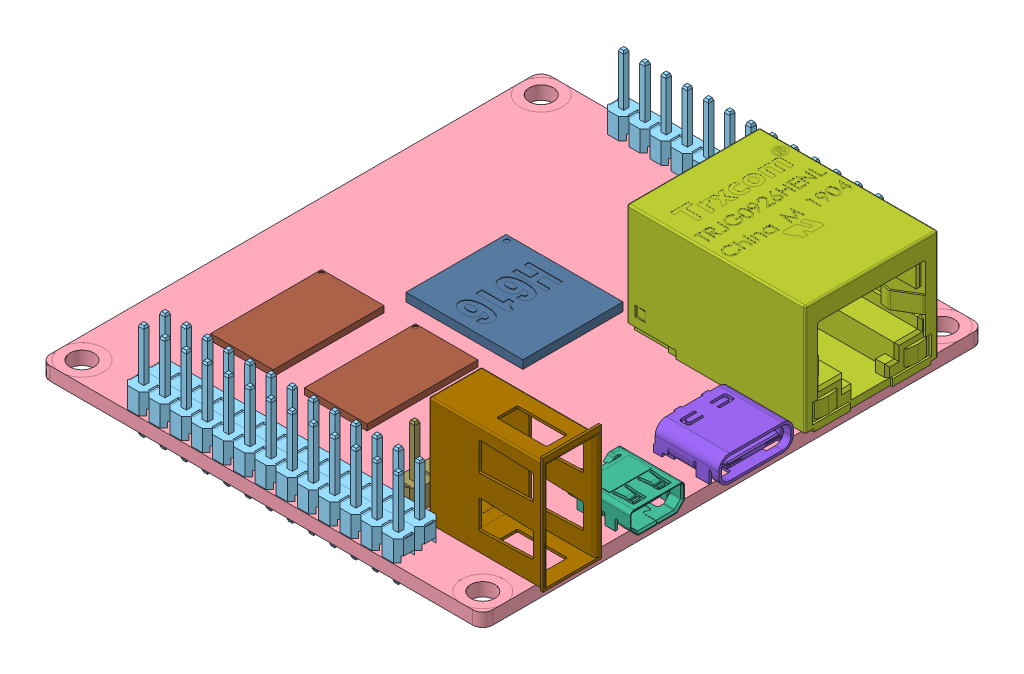
SolidWorks assembly OrangePi_Zero2, configuration 默认. Lengths in mm.
Overall size (54.2 18.1 60).
16 component instances, 12 part files, 37 mates.
Components (placement in the parent):
- Card slot assembly_Domyslna^OrangePi_Zero2-1: Card slot assembly_Domyslna^OrangePi_Zero2 [默认] at (-29.7448 -12.71 -17.6643) x (0 0 -1) z (0 1 0) size (11.95 11.4 1.48) (virtual)
  - card slot part 2 metal pin_Domyslna^Card slot assembly_Domyslna_OrangePi_Zero2-1: card slot part 2 metal pin_Domyslna^Card slot assembly_Domyslna_OrangePi_Zero2 [默认] at (-3.5293 -7.6678 12.2938) x (0 -1 0) z (1 0 0) size (7.95 0.89 8.04) (virtual)
  - sd card slot v1_Domyslna^Card slot assembly_Domyslna_OrangePi_Zero2-1: sd card slot v1_Domyslna^Card slot assembly_Domyslna_OrangePi_Zero2 [默认] at (-18.1743 -9.7848 12.71) x (-1 0 0) z (0 0 -1) size (11.71 10.28 1.3) (virtual)
  - part 3 v1_Domyslna^Card slot assembly_Domyslna_OrangePi_Zero2-1: part 3 v1_Domyslna^Card slot assembly_Domyslna_OrangePi_Zero2 [默认] at (-6.4643 -9.3448 11.38) x (1 0 0) z (0 0 -1) size (11.95 11.4 1.45) (virtual)
- pcb^OrangePi_Zero2-1: pcb^OrangePi_Zero2 [默认] at origin size (53 1.6 60) (virtual)
- PLS-13.step^OrangePi_Zero2-1: PLS-13.step^OrangePi_Zero2 [默认] at (-15.45 1.6 26.09) x (1 0 0) z (0 1 0) size (33.02 2.54 11.6) (virtual)
- PLS-13.step^OrangePi_Zero2-2: PLS-13.step^OrangePi_Zero2 [默认] at (-15.45 1.6 28.63) x (1 0 0) z (0 1 0) size (33.02 2.54 11.6) (virtual)
- PLS-13.step^OrangePi_Zero2-3: PLS-13.step^OrangePi_Zero2 [默认] at (-15.25 1.6 -28.63) x (1 0 0) z (0 1 0) size (33.02 2.54 11.6) (virtual)
- 11.0 Female micro HDMI connector_Domyslna^OrangePi_Zero2-1: 11.0 Female micro HDMI connector_Domyslna^OrangePi_Zero2 [默认] at (20 3.05 10.09) x (0 0 -1) z (1 0 0) size (6.5 3.51 7.5) (virtual)
- 12.0 Gigabit ethernet port raspberry^OrangePi_Zero2-1: 12.0 Gigabit ethernet port raspberry^OrangePi_Zero2 [默认] at (27.3 8.525 -15.75) x (0 0 -1) z (1 0 0) size (16.1 17.2 21.45) (virtual)
- 10.0 Female USB connector_Domyslna^OrangePi_Zero2-1: 10.0 Female USB connector_Domyslna^OrangePi_Zero2 [默认] at (19.99 3.18 -1.63) x (0 0 -1) z (1 0 0) size (8.94 3.96 7.9) (virtual)
- USB-A 111 (vertical on plate)___ _________^OrangePi_Zero2-1: USB-A 111 (vertical on plate)___ _________^OrangePi_Zero2 [默认] at (13.7 8.1368 23.65) x (1 0 0) z (0 1 0) size (14 9.14 18.1) (virtual)
- H616^OrangePi_Zero2-1: H616^OrangePi_Zero2 [默认] at (-3.5 1.72 -3.8) x (0 0 1) z (-1 0 0) size (12 1.12 14) (virtual)
- DDR3^OrangePi_Zero2-1: DDR3^OrangePi_Zero2 [默认] at (-14.25 1.9 11.45) size (7.5 1.03 13.3) (virtual)
- DDR3^OrangePi_Zero2-2: DDR3^OrangePi_Zero2 [默认] at (-3.01 1.9 11.45) size (7.5 1.03 13.3) (virtual)
- PLS-4^OrangePi_Zero2-1: PLS-4^OrangePi_Zero2 [默认] at (10.73 1.6 17.31) x (0 0 1) z (0 1 0) size (7.62 2.54 11.6) (virtual)
Mates (geometry in assembly coordinates):
- 重合1: coincident: plane of pcb^OrangePi_Zero2-1 through (0 1.6 0) normal (0 1 0); plane of 12.0 Gigabit ethernet port raspberry^OrangePi_Zero2-1 through (27.3 1.6 -15.75) normal (0 -1 0)
- 距离1: distance = 0.8 mm: plane of 12.0 Gigabit ethernet port raspberry^OrangePi_Zero2-1 through (27.3 8.525 -15.75) normal (1 0 0); plane of pcb^OrangePi_Zero2-1 through (26.5 1.6 -30) normal (1 0 0)
- 距离2: distance = 6.3 mm: plane of pcb^OrangePi_Zero2-1 through (27.25 1.4 -30) normal (0 0 -1); plane of 12.0 Gigabit ethernet port raspberry^OrangePi_Zero2-1 through (5.95 1.95 -23.7) normal (0 0 -1)
- 重合2: coincident: plane of pcb^OrangePi_Zero2-1 through (0 1.6 0) normal (0 1 0); plane of 10.0 Female USB connector_Domyslna^OrangePi_Zero2-1 through (27.6 1.6 1.54) normal (0 -1 0)
- 距离3: distance = 1.1 mm: plane of 10.0 Female USB connector_Domyslna^OrangePi_Zero2-1 through (27.6 3.46 1.54) normal (1 0 0); plane of pcb^OrangePi_Zero2-1 through (26.5 1.6 -30) normal (1 0 0)
- 距离4: distance = 23.9 mm: plane of pcb^OrangePi_Zero2-1 through (27.25 1.4 -30) normal (0 0 -1); plane of 10.0 Female USB connector_Domyslna^OrangePi_Zero2-1 through (27.6 2.9 -6.1) normal (0 0 -1)
- 重合4: coincident: plane of pcb^OrangePi_Zero2-1 through (0 1.6 0) normal (0 1 0); plane of 11.0 Female micro HDMI connector_Domyslna^OrangePi_Zero2-1 through (22 1.6 7.3221) normal (0 -1 0)
- 重合5: coincident: plane of pcb^OrangePi_Zero2-1 through (0 1.6 0) normal (0 1 0); plane of 11.0 Female micro HDMI connector_Domyslna^OrangePi_Zero2-1 through (22 1.6 7.3221) normal (0 -1 0)
- 距离5: distance = 1 mm: plane of 11.0 Female micro HDMI connector_Domyslna^OrangePi_Zero2-1 through (27.5 2.05 12.2455) normal (1 0 0); plane of pcb^OrangePi_Zero2-1 through (26.5 1.6 -30) normal (1 0 0)
- 距离6: distance = 4 mm: plane of 10.0 Female USB connector_Domyslna^OrangePi_Zero2-1 through (27.6 3.46 2.84) normal (0 0 1); plane of 11.0 Female micro HDMI connector_Domyslna^OrangePi_Zero2-1 through (27.5 2.7298 6.84) normal (0 0 -1)
- 重合7: coincident: plane of pcb^OrangePi_Zero2-1 through (0 1.6 0) normal (0 1 0); plane of USB-A 111 (vertical on plate)___ _________^OrangePi_Zero2-1 through (17.9 1.6 16) normal (0 -1 0)
- 距离7: distance = 1.2 mm: plane of USB-A 111 (vertical on plate)___ _________^OrangePi_Zero2-1 through (27.7 1.5868 17.35) normal (1 0 0); plane of pcb^OrangePi_Zero2-1 through (26.5 1.6 -30) normal (1 0 0)
- 距离8: distance = 6.35 mm: plane of USB-A 111 (vertical on plate)___ _________^OrangePi_Zero2-1 through (13.7 1.5868 23.65) normal (0 0 1); plane of pcb^OrangePi_Zero2-1 through (27.25 1.4 30) normal (0 0 1)
- 重合8: coincident: plane of Card slot assembly_Domyslna^OrangePi_Zero2-1/sd card slot v1_Domyslna^Card slot assembly_Domyslna_OrangePi_Zero2-1 through (-24.6 0 -5.98) normal (0 1 0); plane of pcb^OrangePi_Zero2-1 through (0 0 0) normal (0 -1 0)
- 距离9: distance = 0.4 mm: plane of Card slot assembly_Domyslna^OrangePi_Zero2-1/part 3 v1_Domyslna^Card slot assembly_Domyslna_OrangePi_Zero2-1 through (-26.1 -1.45 -17.175) normal (-1 0 0); plane of pcb^OrangePi_Zero2-1 through (-26.5 1.6 -30) normal (-1 0 0)
- 距离11: distance = 12.825 mm: plane of Card slot assembly_Domyslna^OrangePi_Zero2-1/part 3 v1_Domyslna^Card slot assembly_Domyslna_OrangePi_Zero2-1 through (-26.1 -1.45 -17.175) normal (0 0 -1); plane of pcb^OrangePi_Zero2-1 through (27.25 1.4 -30) normal (0 0 -1)
- 重合11: coincident: plane of pcb^OrangePi_Zero2-1 through (0 1.6 0) normal (0 1 0); plane of PLS-13.step^OrangePi_Zero2-3 through (-12.71 1.6 -28.63) normal (0 -1 0)
- 重合13: coincident: plane of PLS-13.step^OrangePi_Zero2-1 through (-12.91 1.6 26.09) normal (0 -1 0); plane of PLS-13.step^OrangePi_Zero2-2 through (-12.91 1.6 28.63) normal (0 -1 0)
- 重合14: coincident: plane of PLS-13.step^OrangePi_Zero2-1 through (14.36 1.6 27.36) normal (0 0 1); plane of PLS-13.step^OrangePi_Zero2-2 through (15.7 1.6 27.36) normal (0 0 -1)
- 重合15: coincident: plane of PLS-13.step^OrangePi_Zero2-1 through (16.3 1.6 26.76) normal (1 0 0); plane of PLS-13.step^OrangePi_Zero2-2 through (16.3 1.6 29.3) normal (1 0 0)
- 重合16: coincident: plane of pcb^OrangePi_Zero2-1 through (0 1.6 0) normal (0 1 0); plane of PLS-13.step^OrangePi_Zero2-2 through (-12.91 1.6 28.63) normal (0 -1 0)
- 对称1: symmetric: plane of PLS-13.step^OrangePi_Zero2-2 through (14.36 1.6 29.9) normal (0 0 1); plane of PLS-13.step^OrangePi_Zero2-3 through (15.9 1.6 -29.9) normal (0 0 -1); plane of assembly
- 距离12: distance = 59.8 mm: plane of PLS-13.step^OrangePi_Zero2-3 through (15.9 1.6 -29.9) normal (0 0 -1); plane of PLS-13.step^OrangePi_Zero2-2 through (14.36 1.6 29.9) normal (0 0 1)
- 距离13: distance = 10 mm: plane of PLS-13.step^OrangePi_Zero2-3 through (16.5 1.6 -27.96) normal (1 0 0); plane of pcb^OrangePi_Zero2-1 through (26.5 1.6 -30) normal (1 0 0)
- 距离14: distance = 10.2 mm: plane of pcb^OrangePi_Zero2-1 through (26.5 1.6 -30) normal (1 0 0); plane of PLS-13.step^OrangePi_Zero2-2 through (16.3 1.6 29.3) normal (1 0 0)
- 重合17: coincident: plane of pcb^OrangePi_Zero2-1 through (0 1.6 0) normal (0 1 0); plane of PLS-4^OrangePi_Zero2-1 through (10.73 1.6 19.85) normal (0 -1 0)
- 距离15: distance = 6.34 mm: plane of PLS-4^OrangePi_Zero2-1 through (9.46 -1.4 23.66) normal (0 0 1); plane of pcb^OrangePi_Zero2-1 through (27.25 1.4 30) normal (0 0 1)
- 距离16: distance = 14.5 mm: plane of pcb^OrangePi_Zero2-1 through (26.5 1.6 -30) normal (1 0 0); plane of PLS-4^OrangePi_Zero2-1 through (12 1.6 17.98) normal (1 0 0)
- 重合18: coincident: plane of pcb^OrangePi_Zero2-1 through (0 1.6 0) normal (0 1 0); plane of DDR3^OrangePi_Zero2-1 through (-17.445 1.6 17.45) normal (0 -1 0)
- 重合19: coincident: plane of DDR3^OrangePi_Zero2-1 through (-14.25 2.63 11.45) normal (0 1 0); plane of DDR3^OrangePi_Zero2-2 through (-3.01 2.63 11.45) normal (0 1 0)
- 重合20: coincident: plane of DDR3^OrangePi_Zero2-1 through (-10.5 2.63 4.8) normal (0 0 -1); plane of DDR3^OrangePi_Zero2-2 through (0.74 2.63 4.8) normal (0 0 -1)
- 距离17: distance = 3.74 mm: plane of DDR3^OrangePi_Zero2-2 through (-6.76 2.63 18.1) normal (-1 0 0); plane of DDR3^OrangePi_Zero2-1 through (-10.5 2.63 18.1) normal (1 0 0)
- 距离18: distance = 8.5 mm: plane of DDR3^OrangePi_Zero2-1 through (-18 2.63 18.1) normal (-1 0 0); plane of pcb^OrangePi_Zero2-1 through (-26.5 1.6 -30) normal (-1 0 0)
- 距离19: distance = 11.9 mm: plane of DDR3^OrangePi_Zero2-1 through (-10.5 2.63 18.1) normal (0 0 1); plane of pcb^OrangePi_Zero2-1 through (27.25 1.4 30) normal (0 0 1)
- 重合24: coincident: plane of pcb^OrangePi_Zero2-1 through (0 1.6 0) normal (0 1 0); plane of H616^OrangePi_Zero2-1 through (-9.975 1.6 1.7) normal (0 -1 0)
- 距离20: distance = 16 mm: plane of H616^OrangePi_Zero2-1 through (-10.5 2.72 2.2) normal (-1 0 0); plane of pcb^OrangePi_Zero2-1 through (-26.5 1.6 -30) normal (-1 0 0)
- 距离21: distance = 2.6 mm: plane of H616^OrangePi_Zero2-1 through (-10.5 2.72 2.2) normal (0 0 1); plane of DDR3^OrangePi_Zero2-1 through (-10.5 2.63 4.8) normal (0 0 -1)
